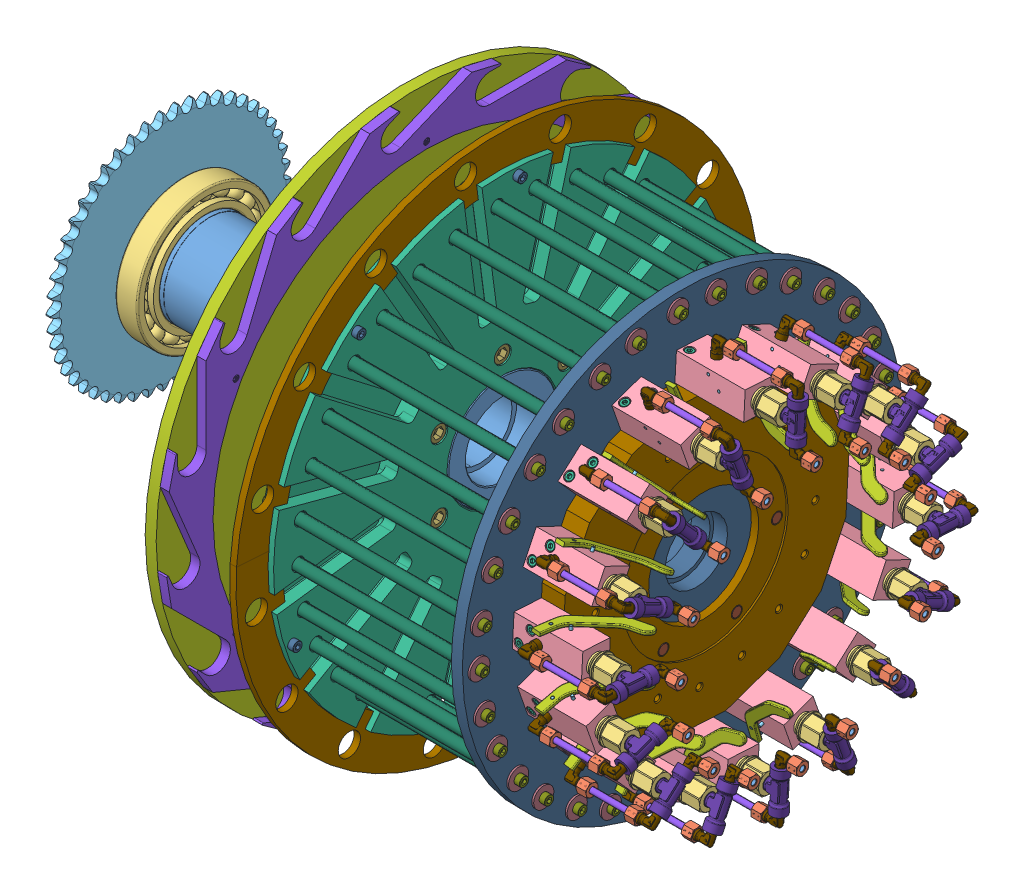
SolidWorks assembly assieme parte rotante, configuration Default. Lengths in mm. (continued)
Components (placement in the parent): (continued)
- AssiemeValvola-7: AssiemeValvola [Default] at (515.3257 -134.8578 488.6421) x (0 0.901303 -0.433189) z (0 -0.433189 -0.901303) size (90.26 138.63 38)
  - RaccordoT-1: RaccordoT [Default] at origin size (43 29.75 16.5)
  - Raccordo a L-1: Raccordo a L [Default] at (-30 0 0) x (0 -1 0) z (0 0 -1) size (28.34 25.51 14.01)
    - 1809_06_10_01-1: 1809_06_10_01 [Default] at origin size (22.49 23 10)
    - 1809_06_10_02-1: 1809_06_10_02 [Default] at origin size (6.5 8.5 8.5)
    - 1809_06_10_03-1: 1809_06_10_03 [Default] at origin size (11.02 15.01 14.01)
  - Raccordo a L-2: Raccordo a L [Default] at (30 0 0) x (0 1 0) z (0 0 -1) size (28.34 25.51 14.01)
    - 1809_06_10_01-1: 1809_06_10_01 [Default] at origin size (22.49 23 10)
    - 1809_06_10_02-1: 1809_06_10_02 [Default] at origin size (6.5 8.5 8.5)
    - 1809_06_10_03-1: 1809_06_10_03 [Default] at origin size (11.02 15.01 14.01)
  - TappoChiusura-1: TappoChiusura [Default] at (0 -32 0) x (0 -1 0) z (0 0 1) size (38.28 26.74 26.74)
  - CorpoValvola-1: CorpoValvola [Default] at (-15 -115.2824 0) size (30 75 34)
  - Raccordo a L-3: Raccordo a L [Default] at (-30 -88.2824 0) x (0 1 0) z (0 0 1) size (28.34 25.51 14.01)
    - 1809_06_10_01-1: 1809_06_10_01 [Default] at origin size (22.49 23 10)
    - 1809_06_10_02-1: 1809_06_10_02 [Default] at origin size (6.5 8.5 8.5)
    - 1809_06_10_03-1: 1809_06_10_03 [Default] at origin size (11.02 15.01 14.01)
  - Spina_3x38-1: Spina_3x38 [Default] at (0 -68.2824 -21) x (-1 0 0) z (0 0 1) size (3 3 38)
  - Spina_3x38-2: Spina_3x38 [Default] at (-10 -80.2824 -21) x (0.996193 0.087174 0) z (0 0 1) size (3 3 38)
  - M5 40mm-3: M5 40mm [ISO 4762 M5 x 40 - 40N] at (-14.6 -108.7824 9) size (45 8.5 8.5)
  - M5 40mm-2: M5 40mm [ISO 4762 M5 x 40 - 40N] at (-14.6 -96.7824 -9) size (45 8.5 8.5)
  - LevaValvola-1: LevaValvola [Default] at (-24.507 -86.571 -17) x (0.996193 0.087174 0) z (0 0 1) size (77.55 60.2 4)
  - Tubo-1: Tubo [Default] at (-30 -15.9665 0) x (1 0 0) z (0 -1 0) size (6 6 56.4)
- AssiemeValvola-8: AssiemeValvola [Default] at (515.3257 -95.0129 541.6718) x (0 0.666921 -0.745128) z (0 -0.745128 -0.666921) size (90.26 138.63 38)
  - RaccordoT-1: RaccordoT [Default] at origin size (43 29.75 16.5)
  - Raccordo a L-1: Raccordo a L [Default] at (-30 0 0) x (0 -1 0) z (0 0 -1) size (28.34 25.51 14.01)
    - 1809_06_10_01-1: 1809_06_10_01 [Default] at origin size (22.49 23 10)
    - 1809_06_10_02-1: 1809_06_10_02 [Default] at origin size (6.5 8.5 8.5)
    - 1809_06_10_03-1: 1809_06_10_03 [Default] at origin size (11.02 15.01 14.01)
  - Raccordo a L-2: Raccordo a L [Default] at (30 0 0) x (0 1 0) z (0 0 -1) size (28.34 25.51 14.01)
    - 1809_06_10_01-1: 1809_06_10_01 [Default] at origin size (22.49 23 10)
    - 1809_06_10_02-1: 1809_06_10_02 [Default] at origin size (6.5 8.5 8.5)
    - 1809_06_10_03-1: 1809_06_10_03 [Default] at origin size (11.02 15.01 14.01)
  - TappoChiusura-1: TappoChiusura [Default] at (0 -32 0) x (0 -1 0) z (0 0 1) size (38.28 26.74 26.74)
  - CorpoValvola-1: CorpoValvola [Default] at (-15 -115.2824 0) size (30 75 34)
  - Raccordo a L-3: Raccordo a L [Default] at (-30 -88.2824 0) x (0 1 0) z (0 0 1) size (28.34 25.51 14.01)
    - 1809_06_10_01-1: 1809_06_10_01 [Default] at origin size (22.49 23 10)
    - 1809_06_10_02-1: 1809_06_10_02 [Default] at origin size (6.5 8.5 8.5)
    - 1809_06_10_03-1: 1809_06_10_03 [Default] at origin size (11.02 15.01 14.01)
  - Spina_3x38-1: Spina_3x38 [Default] at (0 -68.2824 -21) x (-1 0 0) z (0 0 1) size (3 3 38)
  - Spina_3x38-2: Spina_3x38 [Default] at (-10 -80.2824 -21) x (0.996193 0.087174 0) z (0 0 1) size (3 3 38)
  - M5 40mm-3: M5 40mm [ISO 4762 M5 x 40 - 40N] at (-14.6 -108.7824 9) size (45 8.5 8.5)
  - M5 40mm-2: M5 40mm [ISO 4762 M5 x 40 - 40N] at (-14.6 -96.7824 -9) size (45 8.5 8.5)
  - LevaValvola-1: LevaValvola [Default] at (-24.507 -86.571 -17) x (0.996193 0.087174 0) z (0 0 1) size (77.55 60.2 4)
  - Tubo-1: Tubo [Default] at (-30 -15.9665 0) x (1 0 0) z (0 -1 0) size (6 6 56.4)
- AssiemeValvola-9: AssiemeValvola [Default] at (515.3257 -37.9074 575.4168) x (0 0.331007 -0.943628) z (0 -0.943628 -0.331007) size (90.26 138.63 38)
  - RaccordoT-1: RaccordoT [Default] at origin size (43 29.75 16.5)
  - Raccordo a L-1: Raccordo a L [Default] at (-30 0 0) x (0 -1 0) z (0 0 -1) size (28.34 25.51 14.01)
    - 1809_06_10_01-1: 1809_06_10_01 [Default] at origin size (22.49 23 10)
    - 1809_06_10_02-1: 1809_06_10_02 [Default] at origin size (6.5 8.5 8.5)
    - 1809_06_10_03-1: 1809_06_10_03 [Default] at origin size (11.02 15.01 14.01)
  - Raccordo a L-2: Raccordo a L [Default] at (30 0 0) x (0 1 0) z (0 0 -1) size (28.34 25.51 14.01)
    - 1809_06_10_01-1: 1809_06_10_01 [Default] at origin size (22.49 23 10)
    - 1809_06_10_02-1: 1809_06_10_02 [Default] at origin size (6.5 8.5 8.5)
    - 1809_06_10_03-1: 1809_06_10_03 [Default] at origin size (11.02 15.01 14.01)
  - TappoChiusura-1: TappoChiusura [Default] at (0 -32 0) x (0 -1 0) z (0 0 1) size (38.28 26.74 26.74)
  - CorpoValvola-1: CorpoValvola [Default] at (-15 -115.2824 0) size (30 75 34)
  - Raccordo a L-3: Raccordo a L [Default] at (-30 -88.2824 0) x (0 1 0) z (0 0 1) size (28.34 25.51 14.01)
    - 1809_06_10_01-1: 1809_06_10_01 [Default] at origin size (22.49 23 10)
    - 1809_06_10_02-1: 1809_06_10_02 [Default] at origin size (6.5 8.5 8.5)
    - 1809_06_10_03-1: 1809_06_10_03 [Default] at origin size (11.02 15.01 14.01)
  - Spina_3x38-1: Spina_3x38 [Default] at (0 -68.2824 -21) x (-1 0 0) z (0 0 1) size (3 3 38)
  - Spina_3x38-2: Spina_3x38 [Default] at (-10 -80.2824 -21) x (0.996193 0.087174 0) z (0 0 1) size (3 3 38)
  - M5 40mm-3: M5 40mm [ISO 4762 M5 x 40 - 40N] at (-14.6 -108.7824 9) size (45 8.5 8.5)
  - M5 40mm-2: M5 40mm [ISO 4762 M5 x 40 - 40N] at (-14.6 -96.7824 -9) size (45 8.5 8.5)
  - LevaValvola-1: LevaValvola [Default] at (-24.507 -86.571 -17) x (0.996193 0.087174 0) z (0 0 1) size (77.55 60.2 4)
  - Tubo-1: Tubo [Default] at (-30 -15.9665 0) x (1 0 0) z (0 -1 0) size (6 6 56.4)
- AssiemeValvola-10: AssiemeValvola [Default] at (515.3257 27.7648 584.7399) x (0 -0.055301 -0.99847) z (0 -0.99847 0.055301) size (90.26 138.63 38)
  - RaccordoT-1: RaccordoT [Default] at origin size (43 29.75 16.5)
  - Raccordo a L-1: Raccordo a L [Default] at (-30 0 0) x (0 -1 0) z (0 0 -1) size (28.34 25.51 14.01)
    - 1809_06_10_01-1: 1809_06_10_01 [Default] at origin size (22.49 23 10)
    - 1809_06_10_02-1: 1809_06_10_02 [Default] at origin size (6.5 8.5 8.5)
    - 1809_06_10_03-1: 1809_06_10_03 [Default] at origin size (11.02 15.01 14.01)
  - Raccordo a L-2: Raccordo a L [Default] at (30 0 0) x (0 1 0) z (0 0 -1) size (28.34 25.51 14.01)
    - 1809_06_10_01-1: 1809_06_10_01 [Default] at origin size (22.49 23 10)
    - 1809_06_10_02-1: 1809_06_10_02 [Default] at origin size (6.5 8.5 8.5)
    - 1809_06_10_03-1: 1809_06_10_03 [Default] at origin size (11.02 15.01 14.01)
  - TappoChiusura-1: TappoChiusura [Default] at (0 -32 0) x (0 -1 0) z (0 0 1) size (38.28 26.74 26.74)
  - CorpoValvola-1: CorpoValvola [Default] at (-15 -115.2824 0) size (30 75 34)
  - Raccordo a L-3: Raccordo a L [Default] at (-30 -88.2824 0) x (0 1 0) z (0 0 1) size (28.34 25.51 14.01)
    - 1809_06_10_01-1: 1809_06_10_01 [Default] at origin size (22.49 23 10)
    - 1809_06_10_02-1: 1809_06_10_02 [Default] at origin size (6.5 8.5 8.5)
    - 1809_06_10_03-1: 1809_06_10_03 [Default] at origin size (11.02 15.01 14.01)
  - Spina_3x38-1: Spina_3x38 [Default] at (0 -68.2824 -21) x (-1 0 0) z (0 0 1) size (3 3 38)
  - Spina_3x38-2: Spina_3x38 [Default] at (-10 -80.2824 -21) x (0.996193 0.087174 0) z (0 0 1) size (3 3 38)
  - M5 40mm-3: M5 40mm [ISO 4762 M5 x 40 - 40N] at (-14.6 -108.7824 9) size (45 8.5 8.5)
  - M5 40mm-2: M5 40mm [ISO 4762 M5 x 40 - 40N] at (-14.6 -96.7824 -9) size (45 8.5 8.5)
  - LevaValvola-1: LevaValvola [Default] at (-24.507 -86.571 -17) x (0.996193 0.087174 0) z (0 0 1) size (77.55 60.2 4)
  - Tubo-1: Tubo [Default] at (-30 -15.9665 0) x (1 0 0) z (0 -1 0) size (6 6 56.4)
- AssiemeValvola-11: AssiemeValvola [Default] at (515.3257 92.0058 568.2215) x (0 -0.433189 -0.901303) z (0 -0.901303 0.433189) size (90.26 138.63 38)
  - RaccordoT-1: RaccordoT [Default] at origin size (43 29.75 16.5)
  - Raccordo a L-1: Raccordo a L [Default] at (-30 0 0) x (0 -1 0) z (0 0 -1) size (28.34 25.51 14.01)
    - 1809_06_10_01-1: 1809_06_10_01 [Default] at origin size (22.49 23 10)
    - 1809_06_10_02-1: 1809_06_10_02 [Default] at origin size (6.5 8.5 8.5)
    - 1809_06_10_03-1: 1809_06_10_03 [Default] at origin size (11.02 15.01 14.01)
  - Raccordo a L-2: Raccordo a L [Default] at (30 0 0) x (0 1 0) z (0 0 -1) size (28.34 25.51 14.01)
    - 1809_06_10_01-1: 1809_06_10_01 [Default] at origin size (22.49 23 10)
    - 1809_06_10_02-1: 1809_06_10_02 [Default] at origin size (6.5 8.5 8.5)
    - 1809_06_10_03-1: 1809_06_10_03 [Default] at origin size (11.02 15.01 14.01)
  - TappoChiusura-1: TappoChiusura [Default] at (0 -32 0) x (0 -1 0) z (0 0 1) size (38.28 26.74 26.74)
  - CorpoValvola-1: CorpoValvola [Default] at (-15 -115.2824 0) size (30 75 34)
  - Raccordo a L-3: Raccordo a L [Default] at (-30 -88.2824 0) x (0 1 0) z (0 0 1) size (28.34 25.51 14.01)
    - 1809_06_10_01-1: 1809_06_10_01 [Default] at origin size (22.49 23 10)
    - 1809_06_10_02-1: 1809_06_10_02 [Default] at origin size (6.5 8.5 8.5)
    - 1809_06_10_03-1: 1809_06_10_03 [Default] at origin size (11.02 15.01 14.01)
  - Spina_3x38-1: Spina_3x38 [Default] at (0 -68.2824 -21) x (-1 0 0) z (0 0 1) size (3 3 38)
  - Spina_3x38-2: Spina_3x38 [Default] at (-10 -80.2824 -21) x (0.996193 0.087174 0) z (0 0 1) size (3 3 38)
  - M5 40mm-3: M5 40mm [ISO 4762 M5 x 40 - 40N] at (-14.6 -108.7824 9) size (45 8.5 8.5)
  - M5 40mm-2: M5 40mm [ISO 4762 M5 x 40 - 40N] at (-14.6 -96.7824 -9) size (45 8.5 8.5)
  - LevaValvola-1: LevaValvola [Default] at (-24.507 -86.571 -17) x (0.996193 0.087174 0) z (0 0 1) size (77.55 60.2 4)
  - Tubo-1: Tubo [Default] at (-30 -15.9665 0) x (1 0 0) z (0 -1 0) size (6 6 56.4)
- AssiemeValvola-12: AssiemeValvola [Default] at (515.3257 145.0355 528.3766) x (0 -0.745128 -0.666921) z (0 -0.666921 0.745128) size (90.26 138.63 38)
  - RaccordoT-1: RaccordoT [Default] at origin size (43 29.75 16.5)
  - Raccordo a L-1: Raccordo a L [Default] at (-30 0 0) x (0 -1 0) z (0 0 -1) size (28.34 25.51 14.01)
    - 1809_06_10_01-1: 1809_06_10_01 [Default] at origin size (22.49 23 10)
    - 1809_06_10_02-1: 1809_06_10_02 [Default] at origin size (6.5 8.5 8.5)
    - 1809_06_10_03-1: 1809_06_10_03 [Default] at origin size (11.02 15.01 14.01)
  - Raccordo a L-2: Raccordo a L [Default] at (30 0 0) x (0 1 0) z (0 0 -1) size (28.34 25.51 14.01)
    - 1809_06_10_01-1: 1809_06_10_01 [Default] at origin size (22.49 23 10)
    - 1809_06_10_02-1: 1809_06_10_02 [Default] at origin size (6.5 8.5 8.5)
    - 1809_06_10_03-1: 1809_06_10_03 [Default] at origin size (11.02 15.01 14.01)
  - TappoChiusura-1: TappoChiusura [Default] at (0 -32 0) x (0 -1 0) z (0 0 1) size (38.28 26.74 26.74)
  - CorpoValvola-1: CorpoValvola [Default] at (-15 -115.2824 0) size (30 75 34)
  - Raccordo a L-3: Raccordo a L [Default] at (-30 -88.2824 0) x (0 1 0) z (0 0 1) size (28.34 25.51 14.01)
    - 1809_06_10_01-1: 1809_06_10_01 [Default] at origin size (22.49 23 10)
    - 1809_06_10_02-1: 1809_06_10_02 [Default] at origin size (6.5 8.5 8.5)
    - 1809_06_10_03-1: 1809_06_10_03 [Default] at origin size (11.02 15.01 14.01)
  - Spina_3x38-1: Spina_3x38 [Default] at (0 -68.2824 -21) x (-1 0 0) z (0 0 1) size (3 3 38)
  - Spina_3x38-2: Spina_3x38 [Default] at (-10 -80.2824 -21) x (0.996193 0.087174 0) z (0 0 1) size (3 3 38)
  - M5 40mm-3: M5 40mm [ISO 4762 M5 x 40 - 40N] at (-14.6 -108.7824 9) size (45 8.5 8.5)
  - M5 40mm-2: M5 40mm [ISO 4762 M5 x 40 - 40N] at (-14.6 -96.7824 -9) size (45 8.5 8.5)
  - LevaValvola-1: LevaValvola [Default] at (-24.507 -86.571 -17) x (0.996193 0.087174 0) z (0 0 1) size (77.55 60.2 4)
  - Tubo-1: Tubo [Default] at (-30 -15.9665 0) x (1 0 0) z (0 -1 0) size (6 6 56.4)
- AssiemeValvola-13: AssiemeValvola [Default] at (515.3257 178.7805 471.2711) x (0 -0.943628 -0.331007) z (0 -0.331007 0.943628) size (90.26 138.63 38)
  - RaccordoT-1: RaccordoT [Default] at origin size (43 29.75 16.5)
  - Raccordo a L-1: Raccordo a L [Default] at (-30 0 0) x (0 -1 0) z (0 0 -1) size (28.34 25.51 14.01)
    - 1809_06_10_01-1: 1809_06_10_01 [Default] at origin size (22.49 23 10)
    - 1809_06_10_02-1: 1809_06_10_02 [Default] at origin size (6.5 8.5 8.5)
    - 1809_06_10_03-1: 1809_06_10_03 [Default] at origin size (11.02 15.01 14.01)
  - Raccordo a L-2: Raccordo a L [Default] at (30 0 0) x (0 1 0) z (0 0 -1) size (28.34 25.51 14.01)
    - 1809_06_10_01-1: 1809_06_10_01 [Default] at origin size (22.49 23 10)
    - 1809_06_10_02-1: 1809_06_10_02 [Default] at origin size (6.5 8.5 8.5)
    - 1809_06_10_03-1: 1809_06_10_03 [Default] at origin size (11.02 15.01 14.01)
  - TappoChiusura-1: TappoChiusura [Default] at (0 -32 0) x (0 -1 0) z (0 0 1) size (38.28 26.74 26.74)
  - CorpoValvola-1: CorpoValvola [Default] at (-15 -115.2824 0) size (30 75 34)
  - Raccordo a L-3: Raccordo a L [Default] at (-30 -88.2824 0) x (0 1 0) z (0 0 1) size (28.34 25.51 14.01)
    - 1809_06_10_01-1: 1809_06_10_01 [Default] at origin size (22.49 23 10)
    - 1809_06_10_02-1: 1809_06_10_02 [Default] at origin size (6.5 8.5 8.5)
    - 1809_06_10_03-1: 1809_06_10_03 [Default] at origin size (11.02 15.01 14.01)
  - Spina_3x38-1: Spina_3x38 [Default] at (0 -68.2824 -21) x (-1 0 0) z (0 0 1) size (3 3 38)
  - Spina_3x38-2: Spina_3x38 [Default] at (-10 -80.2824 -21) x (0.996193 0.087174 0) z (0 0 1) size (3 3 38)
  - M5 40mm-3: M5 40mm [ISO 4762 M5 x 40 - 40N] at (-14.6 -108.7824 9) size (45 8.5 8.5)
  - M5 40mm-2: M5 40mm [ISO 4762 M5 x 40 - 40N] at (-14.6 -96.7824 -9) size (45 8.5 8.5)
  - LevaValvola-1: LevaValvola [Default] at (-24.507 -86.571 -17) x (0.996193 0.087174 0) z (0 0 1) size (77.55 60.2 4)
  - Tubo-1: Tubo [Default] at (-30 -15.9665 0) x (1 0 0) z (0 -1 0) size (6 6 56.4)
- AssiemeValvola-14: AssiemeValvola [Default] at (515.3257 188.1036 405.5989) x (0 -0.99847 0.055301) z (0 0.055301 0.99847) size (90.26 138.63 38)
  - RaccordoT-1: RaccordoT [Default] at origin size (43 29.75 16.5)
  - Raccordo a L-1: Raccordo a L [Default] at (-30 0 0) x (0 -1 0) z (0 0 -1) size (28.34 25.51 14.01)
    - 1809_06_10_01-1: 1809_06_10_01 [Default] at origin size (22.49 23 10)
    - 1809_06_10_02-1: 1809_06_10_02 [Default] at origin size (6.5 8.5 8.5)
    - 1809_06_10_03-1: 1809_06_10_03 [Default] at origin size (11.02 15.01 14.01)
  - Raccordo a L-2: Raccordo a L [Default] at (30 0 0) x (0 1 0) z (0 0 -1) size (28.34 25.51 14.01)
    - 1809_06_10_01-1: 1809_06_10_01 [Default] at origin size (22.49 23 10)
    - 1809_06_10_02-1: 1809_06_10_02 [Default] at origin size (6.5 8.5 8.5)
    - 1809_06_10_03-1: 1809_06_10_03 [Default] at origin size (11.02 15.01 14.01)
  - TappoChiusura-1: TappoChiusura [Default] at (0 -32 0) x (0 -1 0) z (0 0 1) size (38.28 26.74 26.74)
  - CorpoValvola-1: CorpoValvola [Default] at (-15 -115.2824 0) size (30 75 34)
  - Raccordo a L-3: Raccordo a L [Default] at (-30 -88.2824 0) x (0 1 0) z (0 0 1) size (28.34 25.51 14.01)
    - 1809_06_10_01-1: 1809_06_10_01 [Default] at origin size (22.49 23 10)
    - 1809_06_10_02-1: 1809_06_10_02 [Default] at origin size (6.5 8.5 8.5)
    - 1809_06_10_03-1: 1809_06_10_03 [Default] at origin size (11.02 15.01 14.01)
  - Spina_3x38-1: Spina_3x38 [Default] at (0 -68.2824 -21) x (-1 0 0) z (0 0 1) size (3 3 38)
  - Spina_3x38-2: Spina_3x38 [Default] at (-10 -80.2824 -21) x (0.996193 0.087174 0) z (0 0 1) size (3 3 38)
  - M5 40mm-3: M5 40mm [ISO 4762 M5 x 40 - 40N] at (-14.6 -108.7824 9) size (45 8.5 8.5)
  - M5 40mm-2: M5 40mm [ISO 4762 M5 x 40 - 40N] at (-14.6 -96.7824 -9) size (45 8.5 8.5)
  - LevaValvola-1: LevaValvola [Default] at (-24.507 -86.571 -17) x (0.996193 0.087174 0) z (0 0 1) size (77.55 60.2 4)
  - Tubo-1: Tubo [Default] at (-30 -15.9665 0) x (1 0 0) z (0 -1 0) size (6 6 56.4)
- AssiemeValvola-15: AssiemeValvola [Default] at (515.3257 171.5852 341.3579) x (0 -0.901303 0.433189) z (0 0.433189 0.901303) size (90.26 138.63 38)
  - RaccordoT-1: RaccordoT [Default] at origin size (43 29.75 16.5)
  - Raccordo a L-1: Raccordo a L [Default] at (-30 0 0) x (0 -1 0) z (0 0 -1) size (28.34 25.51 14.01)
    - 1809_06_10_01-1: 1809_06_10_01 [Default] at origin size (22.49 23 10)
    - 1809_06_10_02-1: 1809_06_10_02 [Default] at origin size (6.5 8.5 8.5)
    - 1809_06_10_03-1: 1809_06_10_03 [Default] at origin size (11.02 15.01 14.01)
  - Raccordo a L-2: Raccordo a L [Default] at (30 0 0) x (0 1 0) z (0 0 -1) size (28.34 25.51 14.01)
    - 1809_06_10_01-1: 1809_06_10_01 [Default] at origin size (22.49 23 10)
    - 1809_06_10_02-1: 1809_06_10_02 [Default] at origin size (6.5 8.5 8.5)
    - 1809_06_10_03-1: 1809_06_10_03 [Default] at origin size (11.02 15.01 14.01)
  - TappoChiusura-1: TappoChiusura [Default] at (0 -32 0) x (0 -1 0) z (0 0 1) size (38.28 26.74 26.74)
  - CorpoValvola-1: CorpoValvola [Default] at (-15 -115.2824 0) size (30 75 34)
  - Raccordo a L-3: Raccordo a L [Default] at (-30 -88.2824 0) x (0 1 0) z (0 0 1) size (28.34 25.51 14.01)
    - 1809_06_10_01-1: 1809_06_10_01 [Default] at origin size (22.49 23 10)
    - 1809_06_10_02-1: 1809_06_10_02 [Default] at origin size (6.5 8.5 8.5)
    - 1809_06_10_03-1: 1809_06_10_03 [Default] at origin size (11.02 15.01 14.01)
  - Spina_3x38-1: Spina_3x38 [Default] at (0 -68.2824 -21) x (-1 0 0) z (0 0 1) size (3 3 38)
  - Spina_3x38-2: Spina_3x38 [Default] at (-10 -80.2824 -21) x (0.996193 0.087174 0) z (0 0 1) size (3 3 38)
  - M5 40mm-3: M5 40mm [ISO 4762 M5 x 40 - 40N] at (-14.6 -108.7824 9) size (45 8.5 8.5)
  - M5 40mm-2: M5 40mm [ISO 4762 M5 x 40 - 40N] at (-14.6 -96.7824 -9) size (45 8.5 8.5)
  - LevaValvola-1: LevaValvola [Default] at (-24.507 -86.571 -17) x (0.996193 0.087174 0) z (0 0 1) size (77.55 60.2 4)
  - Tubo-1: Tubo [Default] at (-30 -15.9665 0) x (1 0 0) z (0 -1 0) size (6 6 56.4)
- AssiemeValvola-16: AssiemeValvola [Default] at (515.3257 131.7403 288.3282) x (0 -0.666921 0.745128) z (0 0.745128 0.666921) size (90.26 138.63 38)
  - RaccordoT-1: RaccordoT [Default] at origin size (43 29.75 16.5)
  - Raccordo a L-1: Raccordo a L [Default] at (-30 0 0) x (0 -1 0) z (0 0 -1) size (28.34 25.51 14.01)
    - 1809_06_10_01-1: 1809_06_10_01 [Default] at origin size (22.49 23 10)
    - 1809_06_10_02-1: 1809_06_10_02 [Default] at origin size (6.5 8.5 8.5)
    - 1809_06_10_03-1: 1809_06_10_03 [Default] at origin size (11.02 15.01 14.01)
  - Raccordo a L-2: Raccordo a L [Default] at (30 0 0) x (0 1 0) z (0 0 -1) size (28.34 25.51 14.01)
    - 1809_06_10_01-1: 1809_06_10_01 [Default] at origin size (22.49 23 10)
    - 1809_06_10_02-1: 1809_06_10_02 [Default] at origin size (6.5 8.5 8.5)
    - 1809_06_10_03-1: 1809_06_10_03 [Default] at origin size (11.02 15.01 14.01)
  - TappoChiusura-1: TappoChiusura [Default] at (0 -32 0) x (0 -1 0) z (0 0 1) size (38.28 26.74 26.74)
  - CorpoValvola-1: CorpoValvola [Default] at (-15 -115.2824 0) size (30 75 34)
  - Raccordo a L-3: Raccordo a L [Default] at (-30 -88.2824 0) x (0 1 0) z (0 0 1) size (28.34 25.51 14.01)
    - 1809_06_10_01-1: 1809_06_10_01 [Default] at origin size (22.49 23 10)
    - 1809_06_10_02-1: 1809_06_10_02 [Default] at origin size (6.5 8.5 8.5)
    - 1809_06_10_03-1: 1809_06_10_03 [Default] at origin size (11.02 15.01 14.01)
  - Spina_3x38-1: Spina_3x38 [Default] at (0 -68.2824 -21) x (-1 0 0) z (0 0 1) size (3 3 38)
  - Spina_3x38-2: Spina_3x38 [Default] at (-10 -80.2824 -21) x (0.996193 0.087174 0) z (0 0 1) size (3 3 38)
  - M5 40mm-3: M5 40mm [ISO 4762 M5 x 40 - 40N] at (-14.6 -108.7824 9) size (45 8.5 8.5)
  - M5 40mm-2: M5 40mm [ISO 4762 M5 x 40 - 40N] at (-14.6 -96.7824 -9) size (45 8.5 8.5)
  - LevaValvola-1: LevaValvola [Default] at (-24.507 -86.571 -17) x (0.996193 0.087174 0) z (0 0 1) size (77.55 60.2 4)
  - Tubo-1: Tubo [Default] at (-30 -15.9665 0) x (1 0 0) z (0 -1 0) size (6 6 56.4)
- Disco alimentazione guarnizione fi24.4-1: Disco alimentazione guarnizione fi24.4 [Default] at (198.0433 18.3637 415) x (0 0.065403 0.997859) z (-1 0 0) size (570 285 7.35)
- Disco alimentazione guarnizione fi24.4-2: Disco alimentazione guarnizione fi24.4 [Default] at (198.0433 18.3637 415) x (0 -0.065403 -0.997859) z (-1 0 0) size (570 285 7.35)
- m6 12mm-1: m6 12mm [ISO 4762 M6 x 12 - 12N] at (210.0433 200.6849 574.8914) x (-1 0 0) z (0 0.793353 -0.608761) size (18 10 10)
- m6 12mm-7: m6 12mm [ISO 4762 M6 x 12 - 12N] at (210.0433 260.3445 399.1397) x (-1 0 0) z (0 0.793353 -0.608761) size (18 10 10)
- m6 12mm-8: m6 12mm [ISO 4762 M6 x 12 - 12N] at (210.0433 96.3128 185.3694) x (-1 0 0) z (0 0.793353 -0.608761) size (18 10 10)
- m6 12mm-9: m6 12mm [ISO 4762 M6 x 12 - 12N] at (210.0433 -59.5854 644.6306) x (-1 0 0) z (0 -0.793353 -0.608761) size (18 10 10)
- m6 12mm-10: m6 12mm [ISO 4762 M6 x 12 - 12N] at (210.0433 -223.6171 430.8603) x (-1 0 0) z (0 -0.793353 -0.608761) size (18 10 10)
- m6 12mm-11: m6 12mm [ISO 4762 M6 x 12 - 12N] at (210.0433 -163.9575 255.1086) x (-1 0 0) z (0 0.793353 -0.608761) size (18 10 10)
Mates (geometry in assembly coordinates):
- Concentrico1: concentric anti-aligned: circle of albero rotazione piatti-1; circle of seger 100mm-1
- Coincidente1: coincident anti-aligned: plane of albero rotazione piatti-1 through (-143.4567 18.3637 415) normal (-1 0 0); plane of seger 100mm-1 through (-143.4567 18.3637 415) normal (1 0 0)
- Coincidente2: coincident aligned: plane of albero rotazione piatti-1 through (60.413 18.3637 415) normal (0 1 0); plane of seger 100mm-1 through (-146.4567 18.3637 415) normal (0 1 0)
- Concentrico21: concentric aligned: cylinder of albero rotazione piatti-1 through (60.413 18.3637 415) axis (1 0 0) radius 50; cylinder of SKF - 6020 - 20,DE,NC,20_68-1 through (-152.0942 18.3637 415) axis (1 0 0) radius 50
- Coincidente3: coincident anti-aligned: plane of seger 100mm-1 through (-143.4567 18.3637 415) normal (1 0 0); plane of SKF - 6020 - 20,DE,NC,20_68-1 through (-143.4567 -33.4256 439.9823) normal (-1 0 0)
- Concentrico3: concentric aligned: cylinder of albero rotazione piatti-1 through (60.413 18.3637 415) axis (1 0 0) radius 47.5; cylinder of calettatore d95-1 through (-193.8867 18.3637 415) axis (1 0 0) radius 47.5
- Coincidente7: coincident aligned: plane of albero rotazione piatti-1 through (60.413 18.3637 415) normal (0 1 0); plane of calettatore d95-1 through (-178.8867 18.3637 415) normal (0 1 0)
- Concentrico5: concentric aligned: cylinder of albero rotazione piatti-1 through (60.413 18.3637 415) axis (1 0 0) radius 49.75; cylinder of SKF - 6020 - 20,DE,NC,20_68-2 through (41.4058 18.3637 415) axis (1 0 0) radius 50
- Coincidente8: coincident anti-aligned: plane of albero rotazione piatti-1 through (74.0433 18.3637 415) normal (-1 0 0); plane of SKF - 6020 - 20,DE,NC,20_68-2 through (74.0433 -28.0673 437.2803) normal (1 0 0)
- Concentrico6: concentric aligned: cylinder of albero rotazione piatti-1 through (60.413 18.3637 415) axis (1 0 0) radius 60; cylinder of Disco supporto montaggio e Colonne-1 through (5.3377 18.3637 415) axis (1 0 0) radius 60
- Concentrico7: concentric aligned: cylinder of albero rotazione piatti-1 through (101.3656 98.3637 415) axis (1 0 0) radius 6.25; cylinder of Disco supporto montaggio e Colonne-1 through (204.0433 98.3637 415) axis (1 0 0) radius 9.25
- Coincidente9: coincident anti-aligned: plane of albero rotazione piatti-1 through (175.0433 18.3637 415) normal (1 0 0); plane of Disco supporto montaggio e Colonne-1 through (175.0433 18.3637 415) normal (-1 0 0)
- Concentrico8: concentric anti-aligned: cylinder of albero rotazione piatti-1 through (60.413 18.3637 415) axis (1 0 0) radius 60; cylinder of piatto rotante porta tappi-1 through (111.0433 18.3637 415) axis (-1 0 0) radius 60
- Concentrico9: concentric aligned: circle of albero rotazione piatti-1; circle of piatto rotante porta tappi-1
- Coincidente10: coincident anti-aligned: plane of albero rotazione piatti-1 through (119.0433 18.3637 415) normal (-1 0 0); plane of piatto rotante porta tappi-1 through (119.0433 18.3637 415) normal (1 0 0)
- Concentrico10: concentric aligned: cylinder of piatto rotante porta tappi-1 through (119.0433 18.3637 415) axis (-1 0 0) radius 233; cylinder of disco trasportatore tappi 31-1 through (121.0433 18.3637 415) axis (-1 0 0) radius 233
- Tangente2: tangent: cylinder of piatto rotante porta tappi-1 through (98.5243 -101.6363 622.8461) axis (1 0 0) radius 3.25; curve of disco trasportatore tappi 31-1
- Coincidente13: coincident anti-aligned: plane of piatto rotante porta tappi-1 through (111.0433 18.3637 415) normal (1 0 0); plane of disco trasportatore tappi 31-1 through (111.0433 18.3637 415) normal (-1 0 0)
- Concentrico11: concentric anti-aligned: cylinder of albero rotazione piatti-1 through (60.413 18.3637 415) axis (1 0 0) radius 40; cylinder of disco trascinato porta distributore vuoto-1 through (400.0433 18.3637 415) axis (-1 0 0) radius 30
- Concentrico12: concentric anti-aligned: cylinder of Disco supporto montaggio e Colonne-1 through (204.0433 -202.0247 450.2415) axis (1 0 0) radius 6; cylinder of disco trascinato porta distributore vuoto-1 through (417.0139 -202.0247 450.2415) axis (-1 0 0) radius 6
- Coincidente14: coincident anti-aligned: plane of Distributore Rotante-1 through (400.0433 18.3637 415) normal (-1 0 0); plane of disco trascinato porta distributore vuoto-1 through (400.0433 18.3637 415) normal (1 0 0)
- Concentrico13: concentric anti-aligned: circle of Distributore Rotante-1; circle of disco trascinato porta distributore vuoto-1
- Concentrico14: concentric anti-aligned: cylinder of Distributore Rotante-1 through (230.3377 18.3637 415) axis (1 0 0) radius 60; cylinder of disco trascinato porta distributore vuoto-1 through (415.0433 18.3637 415) axis (-1 0 0) radius 67.5
- Concentrico15: concentric anti-aligned: cylinder of disco trascinato porta distributore vuoto-1 through (388.0433 -53.0243 378.8925) axis (1 0 0) radius 6.25; cylinder of m12 35mm-1 through (344.2933 -53.0243 378.8925) axis (-1 0 0) radius 6
- Coincidente15: coincident anti-aligned: plane of disco trascinato porta distributore vuoto-1 through (388.0433 18.3637 415) normal (-1 0 0); plane of m12 35mm-1 through (388.0433 -45.2301 383.3925) normal (1 0 0)
- Parallelo1: parallel anti-aligned: plane of m12 35mm-1 through (382.0433 -47.9668 381.8125) normal (0 -1 0)
- Concentrico16: concentric aligned: cylinder of Disco supporto montaggio e Colonne-1 through (204.0433 -21.6363 345.718) axis (1 0 0) radius 9.25; cylinder of m12 90mm-3 through (234.7933 -21.6363 345.718) axis (1 0 0) radius 6
- Coincidente17: coincident anti-aligned: plane of Disco supporto montaggio e Colonne-1 through (191.0433 -27.049 342.593) normal (1 0 0); plane of m12 90mm-3 through (191.0433 -29.4305 341.218) normal (-1 0 0)
- Parallelo2: parallel aligned: plane of m12 35mm-1 through (382.0433 -47.9668 381.8125) normal (0 -1 0); plane of m12 90mm-3 through (197.0433 -16.5788 348.6379) normal (0 -1 0)
- Concentrico171: concentric anti-aligned: cylinder of piatto rotante porta tappi-1 through (98.5243 -101.6363 207.1539) axis (1 0 0) radius 3.25; cylinder of rondella m6 22mm-1 through (64.1183 -101.6363 207.1539) axis (-1 0 0) radius 3.3
- Coincidente191: coincident anti-aligned: plane of piatto rotante porta tappi-1 through (99.0433 18.3637 415) normal (-1 0 0); plane of rondella m6 22mm-1 through (99.0433 -101.6363 210.4539) normal (1 0 0)
- Parallelo3: parallel anti-aligned: plane of rondella m6 22mm-1 through (99.0433 -101.6363 207.1539) normal (0 -1 0)
- Concentrico181: concentric aligned: cylinder of rondella m6 22mm-1 through (64.1183 -101.6363 207.1539) axis (-1 0 0) radius 3.3; cylinder of M6 20mm-1 through (59.2933 -101.6363 207.1539) axis (-1 0 0) radius 5
- Coincidente211: coincident anti-aligned: plane of rondella m6 22mm-1 through (97.0433 -101.6363 218.1539) normal (-1 0 0); plane of M6 20mm-1 through (97.0433 -97.3062 204.6539) normal (1 0 0)
- Parallelo4: parallel aligned: plane of m12 35mm-1 through (382.0433 -47.9668 381.8125) normal (0 -0.5 -0.866025); plane of M6 20mm-1 through (94.0433 -101.6363 210.0892) normal (0 -0.5 -0.866025)
- Concentrico19: concentric anti-aligned: cylinder of Disco supporto montaggio e Colonne-1 through (204.0433 70.1437 197.9013) axis (1 0 0) radius 6; cylinder of asta scorrimento carello-1 through (400.0433 70.1437 197.9013) axis (-1 0 0) radius 6
- Concentrico201: concentric aligned: cylinder of asta scorrimento carello-1 through (175.0433 70.1437 197.9013) axis (-1 0 0) radius 3.2; cylinder of rondella m6 22mm-7 through (140.1183 70.1437 197.9013) axis (-1 0 0) radius 3.3
- Coincidente231: coincident anti-aligned: plane of asta scorrimento carello-1 through (175.0433 70.1437 197.9013) normal (-1 0 0); plane of rondella m6 22mm-7 through (175.0433 70.1437 201.2013) normal (1 0 0)
- Concentrico211: concentric aligned: cylinder of rondella m6 22mm-7 through (140.1183 70.1437 197.9013) axis (-1 0 0) radius 3.3; cylinder of M6 16mm-1 through (135.2933 70.1437 197.9013) axis (-1 0 0) radius 5
- Coincidente241: coincident anti-aligned: plane of rondella m6 22mm-7 through (173.0433 70.1437 208.9013) normal (-1 0 0); plane of M6 16mm-1 through (173.0433 75.1437 197.9013) normal (1 0 0)
- Parallelo5: parallel aligned: plane of asta scorrimento carello-1 through (287.5433 70.1437 197.9013) normal (0 0 -1); plane of M6 16mm-1 through (170.0433 68.6761 200.4433) normal (0 0 -1)
- Parallelo9: parallel anti-aligned: plane of rondella m6 22mm-7 through (175.0433 70.1437 197.9013) normal (0 0 1); plane of M6 16mm-1 through (170.0433 68.6761 200.4433) normal (0 0 -1)
- Coincidente30: coincident anti-aligned: plane of Disco supporto montaggio e Colonne-1 through (175.0433 18.3637 415) normal (-1 0 0); plane of rondella m6 22mm-7 through (175.0433 70.1437 201.2013) normal (1 0 0)
- Coincidente31: coincident anti-aligned: plane of disco trascinato porta distributore vuoto-1 through (400.0433 18.3637 415) normal (1 0 0); plane of rondella m6 22mm-8 through (400.0433 70.1437 201.2013) normal (-1 0 0)
- Coincidente32: coincident anti-aligned: plane of Distributore Rotante-1 through (400.0433 40.5763 258.5322) normal (0 0.331007 -0.943628); plane of AssiemeValvola-1/CorpoValvola-1 through (400.0433 85.7114 274.3647) normal (0 -0.331007 0.943628)
- Coincidente33: coincident anti-aligned: plane of disco trascinato porta distributore vuoto-1 through (400.0433 18.3637 415) normal (1 0 0); plane of AssiemeValvola-1/CorpoValvola-1 through (400.0433 95.6416 246.0559) normal (-1 0 0)
- Concentrico22: concentric anti-aligned: cylinder of Distributore Rotante-1 through (412.5433 55.4365 309.3136) axis (0 0.331007 -0.943628) radius 3; cylinder of AssiemeValvola-1/CorpoValvola-1 through (412.5433 69.6697 268.7376) axis (0 -0.331007 0.943628) radius 3
- Concentrico23: concentric anti-aligned: cylinder of Disco supporto montaggio e Colonne-1 through (198.0433 18.3637 415) axis (-1 0 0) radius 235; cylinder of Disco alimentazione guarnizione fi24.4-2 through (191.0433 18.3637 415) axis (1 0 0) radius 235
- Concentrico24: concentric anti-aligned: cylinder of Disco supporto montaggio e Colonne-1 through (198.0433 18.3637 415) axis (-1 0 0) radius 235; cylinder of Disco alimentazione guarnizione fi24.4-1 through (191.0433 18.3637 415) axis (1 0 0) radius 235
- Coincidente34: coincident anti-aligned: plane of Disco alimentazione guarnizione fi24.4-1 through (191.0433 33.7334 649.4968) normal (0 -0.997859 0.065403); plane of Disco alimentazione guarnizione fi24.4-2 through (191.0433 37.0036 699.3898) normal (0 0.997859 -0.065403)
- Coincidente35: coincident aligned: plane of Disco alimentazione guarnizione fi24.4-1 through (198.0433 18.3637 415) normal (1 0 0); plane of Disco alimentazione guarnizione fi24.4-2 through (198.0433 18.3637 415) normal (1 0 0)
- Concentrico25: concentric anti-aligned: cylinder of Disco supporto montaggio e Colonne-1 through (188.8509 -59.5854 644.6306) axis (1 0 0) radius 3.25; circle of Disco alimentazione guarnizione fi24.4-2
- Coincidente36: coincident anti-aligned: plane of Disco supporto montaggio e Colonne-1 through (198.0433 18.3637 415) normal (-1 0 0); plane of Disco alimentazione guarnizione fi24.4-2 through (198.0433 18.3637 415) normal (1 0 0)
- Concentrico26: concentric anti-aligned: cylinder of Disco supporto montaggio e Colonne-1 through (188.8509 200.6849 574.8914) axis (1 0 0) radius 3.25; cylinder of M6 16mm-65 through (198.0564 200.6849 574.8914) axis (-1 0 0) radius 3
- Concentrico271: concentric anti-aligned: cone of Disco supporto montaggio e Colonne-1 through (203.0433 200.6849 574.8914) axis (-1 0 0); cylinder of m6 12mm-1 through (241.7933 200.6849 574.8914) axis (1 0 0) radius 5
- Coincidente381: coincident anti-aligned: plane of Disco supporto montaggio e Colonne-1 through (204.0433 18.3637 415) normal (1 0 0); plane of m6 12mm-1 through (204.0433 203.7287 578.8581) normal (-1 0 0)
- Concentrico281: concentric anti-aligned: cylinder of Disco supporto montaggio e Colonne-1 through (203.0433 260.3445 399.1397) axis (-1 0 0) radius 785.3982; cylinder of m6 12mm-7 through (241.7933 260.3445 399.1397) axis (1 0 0) radius 5
- Coincidente401: coincident anti-aligned: plane of Disco supporto montaggio e Colonne-1 through (204.0433 18.3637 415) normal (1 0 0); plane of m6 12mm-7 through (204.0433 263.3883 403.1065) normal (-1 0 0)
- Parallelo11: parallel aligned: plane of m6 12mm-1 through (207.0433 198.898 572.5627) normal (0 0.92388 0.382683); plane of m6 12mm-7 through (207.0433 258.5576 396.8111) normal (0 0.92388 0.382683)
- Concentrico291: concentric anti-aligned: cylinder of Disco supporto montaggio e Colonne-1 through (203.0433 96.3128 185.3694) axis (-1 0 0) radius 785.3982; cylinder of m6 12mm-8 through (241.7933 96.3128 185.3694) axis (1 0 0) radius 5
- Coincidente421: coincident anti-aligned: plane of Disco supporto montaggio e Colonne-1 through (204.0433 18.3637 415) normal (1 0 0); plane of m6 12mm-8 through (204.0433 99.3566 189.3362) normal (-1 0 0)
- Coincidente44: coincident aligned: plane of m6 12mm-7 through (207.0433 259.2212 401.8516) normal (0 0.793353 -0.608761); plane of m6 12mm-8 through (207.0433 95.1895 188.0813) normal (0 0.793353 -0.608761)
- Concentrico301: concentric anti-aligned: cylinder of Disco supporto montaggio e Colonne-1 through (203.0433 -59.5854 644.6306) axis (-1 0 0) radius 785.3982; cylinder of m6 12mm-9 through (241.7933 -59.5854 644.6306) axis (1 0 0) radius 5
- Coincidente451: coincident anti-aligned: plane of Disco supporto montaggio e Colonne-1 through (204.0433 18.3637 415) normal (1 0 0); plane of m6 12mm-9 through (204.0433 -56.5416 640.6638) normal (-1 0 0)
- Concentrico311: concentric anti-aligned: cylinder of Disco supporto montaggio e Colonne-1 through (203.0433 -223.6171 430.8603) axis (-1 0 0) radius 785.3982; cylinder of m6 12mm-10 through (241.7933 -223.6171 430.8603) axis (1 0 0) radius 5
- Coincidente461: coincident anti-aligned: plane of Disco supporto montaggio e Colonne-1 through (204.0433 18.3637 415) normal (1 0 0); plane of m6 12mm-10 through (204.0433 -220.5733 426.8935) normal (-1 0 0)
- Concentrico321: concentric anti-aligned: cylinder of Disco supporto montaggio e Colonne-1 through (203.0433 -163.9575 255.1086) axis (-1 0 0) radius 785.3982; cylinder of m6 12mm-11 through (241.7933 -163.9575 255.1086) axis (1 0 0) radius 5
- Coincidente471: coincident anti-aligned: plane of Disco supporto montaggio e Colonne-1 through (204.0433 18.3637 415) normal (1 0 0); plane of m6 12mm-11 through (204.0433 -160.9136 259.0754) normal (-1 0 0)
- Parallelo13: parallel aligned: plane of m6 12mm-9 through (207.0433 -62.4955 644.2474) normal (0 0.92388 -0.382683); plane of m6 12mm-10 through (207.0433 -226.5272 430.4771) normal (0 0.92388 -0.382683)
- Parallelo14: parallel aligned: plane of Disco supporto montaggio e Colonne-1 through (191.0433 26.2972 408.9124) normal (0 -0.793353 0.608761); plane of m6 12mm-11 through (207.0433 -162.8342 252.3968) normal (0 -0.793353 0.608761)
- Parallelo15: parallel aligned: plane of Disco supporto montaggio e Colonne-1 through (191.0433 19.669 405.0856) normal (0 -0.130526 0.991445); plane of m6 12mm-10 through (207.0433 -221.8302 428.5316) normal (0 -0.130526 0.991445)
- Concentrico322: concentric anti-aligned: cylinder of albero rotazione piatti-1 through (60.413 18.3637 415) axis (1 0 0) radius 47.5; cylinder of Chain wheel ISO - 50Z 10A-1-1 through (-139.8862 18.3637 415) axis (-1 0 0) radius 47.5
- Coincidente472: coincident anti-aligned: plane of albero rotazione piatti-1 through (-155.9567 18.3637 415) normal (-1 0 0); plane of Chain wheel ISO - 50Z 10A-1-1 through (-155.9567 18.3637 415) normal (1 0 0)
- Concentrico323: concentric anti-aligned: cylinder of calettatore d95-1 through (-190.8867 18.3637 415) axis (1 0 0) radius 67.5; cylinder of Chain wheel ISO - 50Z 10A-1-1 through (-164.8867 18.3637 415) axis (-1 0 0) radius 67.5
- Coincidente473: coincident anti-aligned: plane of calettatore d95-1 through (-164.8867 84.9137 415) normal (1 0 0); plane of Chain wheel ISO - 50Z 10A-1-1 through (-164.8867 18.3637 415) normal (-1 0 0)
- Parallelo16: parallel aligned: plane of Chain wheel ISO - 50Z 10A-1-1 through (-164.8867 18.3637 415) normal (0 1 0)
- Parallelo17: parallel aligned: plane of calettatore d95-1 through (-178.8867 18.3637 415) normal (0 1 0)
